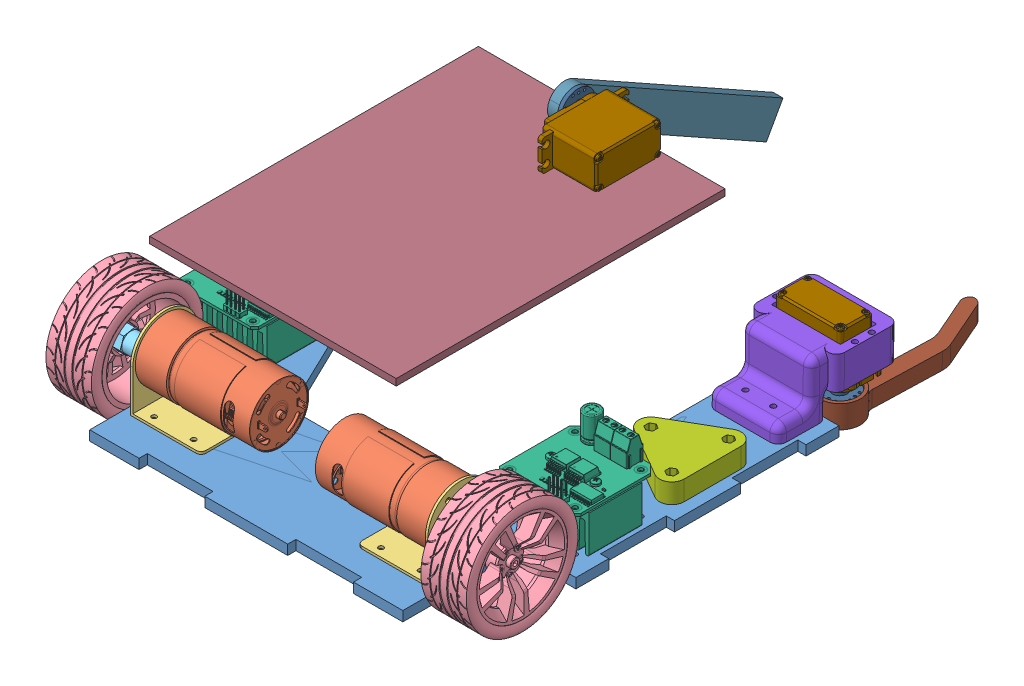
SolidWorks assembly Assem1, configuration Default. Lengths in mm.
Overall size (282.51 155.39 348.37).
30 component instances, 14 part files, 41 mates.
Components (placement in the parent):
- Part2-1: Part2 [Default] at (65.9546 135.2109 209.7386) size (261.02 6 230)
- assemblage_motor_complet-1: assemblage_motor_complet [Default] at (115.1812 215.9173 341.5945) x (0 0 -1) z (-1 0 0) size (92.56 92.56 113.78)
  - Motor 300RPM-1: Motor 300RPM [Default] at (60.9586 47.2064 18.9845) size (37 37 94.88)
  - BAse-motor-1: BAse-motor [Predeterminado] at (28.5836 74.7064 94.3595) x (1 0 0) z (0 0 -1) size (40 46 43)
  - wheel-1: wheel [Default] at (48.5836 55.7064 86.8847) x (-0.872522 -0.488575 0) z (-0.488575 0.872522 0) size (68 29.75 68)
  - accoupelement court-1: accoupelement court [Default] at (48.5836 55.7064 101.8595) x (-0.320714 0.947176 0) z (0 0 1) size (13.86 12 18)
- assemblage_motor_complet-2: assemblage_motor_complet [Default] at (107.4867 215.9173 244.4273) x (0 0 1) z (1 0 0) size (92.56 92.56 113.78)
  - Motor 300RPM-1: Motor 300RPM [Default] at (60.9586 47.2064 18.9845) size (37 37 94.88)
  - BAse-motor-1: BAse-motor [Predeterminado] at (28.5836 74.7064 94.3595) x (1 0 0) z (0 0 -1) size (40 46 43)
  - wheel-1: wheel [Default] at (48.5836 55.7064 86.8847) x (-0.872522 -0.488575 0) z (-0.488575 0.872522 0) size (68 29.75 68)
  - accoupelement court-1: accoupelement court [Default] at (48.5836 55.7064 101.8595) x (-0.320714 0.947176 0) z (0 0 1) size (13.86 12 18)
- IBT-2-module-only-1: IBT-2-module-only [Default] at (209.3463 164.2109 229.8359) size (51 40.62 49.7)
- IBT-2-module-only-4: IBT-2-module-only [Default] at (13.3217 164.5716 229.8359) size (51 40.62 49.7)
- gfg-1: gfg [Défaut] at (217.3463 141.2109 172.8314) x (0.866025 0 0.5) z (-0.5 0 0.866025) size (49.64 15.5 45)
- gfg-2: gfg [Défaut] at (5.3217 141.2109 172.8314) x (0.866025 0 -0.5) z (0.5 0 0.866025) size (49.64 15.5 45)
- support_servo_pince_lamen_isar-1: support_servo_pince_lamen_isar [Default] at (9.3217 155.972 83.8247) x (0 -0.01251 -0.999922) z (0 0.999922 -0.01251) size (68 53 35)
- Part2-2: Part2 [Default] at (65.9546 135.2109 209.7386) size (261.02 6 230)
- support_servo_pince_lamen_isar-2: support_servo_pince_lamen_isar [Default] at (213.3463 155.972 83.8247) x (0 -0.01251 -0.999922) z (0 0.999922 -0.01251) size (68 53 35)
- Servo noir-2: Servo noir [По умолчанию] at (9.3217 182.4699 83.4932) x (1 0 0) z (0 -0.01251 -0.999922) size (53 41.52 20)
- piece de liaison cercle MG996r-3: piece de liaison cercle MG996r [Défaut] at (-0.6783 141.3231 84.008) x (0.979866 0.002498 0.199641) z (0 -0.999922 0.01251) size (20.75 20.75 5.3)
- pince lamen-2: pince lamen [Default] at (-0.6783 134.0237 84.0993) x (0.02377 -0.012506 -0.999639) z (0 0.999922 -0.01251) size (105.33 28.11 13.75)
- Servo noir-3: Servo noir [По умолчанию] at (213.3463 182.4699 83.4932) x (-1 0 0) z (0 0.01251 0.999922) size (53 41.52 20)
- piece de liaison cercle MG996r-4: piece de liaison cercle MG996r [Défaut] at (223.3463 141.3231 84.008) x (-0.987212 0.001994 0.159399) z (0 -0.999922 0.01251) size (20.75 20.75 5.3)
- pince lamen-3: pince lamen [Default] at (223.3463 134.0237 84.0993) x (0.017139 -0.012508 -0.999775) z (0 -0.999922 0.01251) size (105.33 28.11 13.75)
- BillePorteuse-1: BillePorteuse [Défaut] at (5.3217 135.7109 172.8314) x (-1 0 0) z (0 0 1) size (31 21.5 31)
- BillePorteuse-2: BillePorteuse [Défaut] at (217.3463 135.7109 172.8314) x (-1 0 0) z (0 0 1) size (31 21.5 31)
- etage-1: etage [Default] at (111.334 241.2109 216.8002) x (0 0 -1) z (0 1 0) size (200 150 4)
- Servo noir-4: Servo noir [По умолчанию] at (150.296 255.2109 139.0433) x (0 0 1) z (0 -1 0) size (53 41.52 20)
- pince-1: pince [Default] at (100.996 223.6233 72.6584) x (0 -0.488677 -0.872465) z (1 0 0) size (150 20.75 6)
- piece de liaison cercle MG996r-5: piece de liaison cercle MG996r [Défaut] at (109.296 255.2109 129.0433) x (0 0.998874 -0.047442) z (-1 0 0) size (20.75 20.75 5.3)
Mates (geometry in assembly coordinates):
- Coincident5: coincident anti-aligned: plane of Part2-1 through (65.9546 141.2109 209.7386) normal (0 1 0); plane of assemblage_motor_complet-1/BAse motor-1 through (22.3217 141.2109 313.0109) normal (0 -1 0)
- Distance2: distance = 40 mm aligned: plane of Part2-1 through (-19.1783 141.2109 133.0109) normal (-1 0 0); plane of assemblage_motor_complet-1/BAse motor-1 through (20.8217 167.2109 293.0109) normal (-1 0 0)
- Distance1: distance = 20 mm aligned: plane of assemblage_motor_complet-1/BAse motor-1 through (22.3217 141.2109 313.0109) normal (0 0 1); plane of Part2-1 through (-19.1783 141.2109 333.0109) normal (0 0 1)
- Distance3: distance = 7 mm aligned: plane of IBT-2 (module only)-1 through (234.8463 164.2109 248.0109) normal (1 0 0); plane of Part2-1 through (241.8463 141.2109 133.0109) normal (1 0 0)
- Distance4: distance = 15 mm aligned: plane of IBT-2 (module only)-1 through (209.3463 164.2109 248.0109) normal (0 0 1); plane of Part2-1 through (65.9546 131.2109 263.0109) normal (0 0 1)
- Coincident12: coincident: plane of Part2-1 through (65.9546 141.2109 209.7386) normal (0 1 0); point of IBT-2 (module only)-1
- Distance5: distance = 7 mm aligned: plane of IBT-2 (module only)-4 through (-12.1783 164.5716 248.0109) normal (-1 0 0); plane of Part2-1 through (-19.1783 141.2109 133.0109) normal (-1 0 0)
- Distance6: distance = 15 mm aligned: plane of IBT-2 (module only)-4 through (13.3217 164.5716 248.0109) normal (0 0 1); plane of Part2-1 through (-19.1783 131.2109 263.0109) normal (0 0 1)
- Distance10: distance = 7 mm aligned: plane of gfg-1 through (234.8463 153.2109 155.5109) normal (1 0 0); plane of Part2-1 through (241.8463 141.2109 133.0109) normal (1 0 0)
- Distance11: distance = 45 mm: cylinder of gfg-1 through (227.3463 153.2109 155.5109) axis (0 -1 0) radius 7.5; plane of Part2-1 through (65.9546 135.2109 103.0109) normal (0 0 -1)
- Coincident24: coincident anti-aligned: plane of Servo noir-1 through (-18.4913 420.0414 279.4883) normal (0 0 1); plane of support_servo_pince_lamen_isar-3 through (-10.8029 395.353 279.4883) normal (0 0 -1)
- Width1: width anti-aligned: plane of Servo noir-1 through (-20.8029 413.353 273.4883) normal (-1 0 0); plane of Servo noir-1 through (-0.8029 413.353 273.4883) normal (1 0 0); plane of support_servo_pince_lamen_isar-3 through (-21.8029 374.353 299.4883) normal (1 0 0); plane of support_servo_pince_lamen_isar-3 through (0.1971 374.353 299.4883) normal (-1 0 0)
- Coincident29: coincident aligned: circle of Servo noir-2; circle of piece de liaison cercle MG996r-3
- Coincident30: coincident anti-aligned: plane of support_servo_pince_lamen_isar-1 through (9.3217 155.972 83.8247) normal (0 -0.999922 0.01251); plane of Servo noir-2 through (-15.3667 156.0682 91.5125) normal (0 0.999922 -0.01251)
- Coincident31: coincident aligned: circle of piece de liaison cercle MG996r-3; circle of pince lamen-2
- Coincident32: coincident aligned: circle of piece de liaison cercle MG996r-3; circle of pince lamen-2
- Concentric10: concentric aligned: circle of support_servo_pince_lamen_isar-1; circle of Servo noir-2
- Concentric11: concentric aligned: circle of support_servo_pince_lamen_isar-1; circle of Servo noir-2
- Concentric12: concentric aligned: circle of support_servo_pince_lamen_isar-2; circle of Servo noir-3
- Concentric13: concentric aligned: circle of support_servo_pince_lamen_isar-2; circle of Servo noir-3
- Coincident33: coincident anti-aligned: plane of support_servo_pince_lamen_isar-2 through (213.3463 155.972 83.8247) normal (0 -0.999922 0.01251); plane of Servo noir-3 through (238.0347 155.8758 76.1369) normal (0 0.999922 -0.01251)
- Coincident35: coincident aligned: circle of Servo noir-3; circle of piece de liaison cercle MG996r-4
- Coincident36: coincident anti-aligned: circle of piece de liaison cercle MG996r-4; circle of pince lamen-3
- Coincident37: coincident anti-aligned: circle of piece de liaison cercle MG996r-4; circle of pince lamen-3
- Distance12: distance = 7 mm aligned: plane of support_servo_pince_lamen_isar-1 through (-12.1783 176.5834 132.5707) normal (-1 0 0); plane of Part2-1 through (-19.1783 141.2109 133.0109) normal (-1 0 0)
- Distance13: distance = 0 mm: line of support_servo_pince_lamen_isar-1 through (-7.1783 141.2109 103.0109) axis (1 0 0); line of Part2-2 through (-19.1783 141.2109 103.0109) axis (1 0 0)
- Coincident41: coincident anti-aligned: plane of Part2-1 through (65.9546 141.2109 209.7386) normal (0 1 0); plane of gfg-1 through (227.3463 141.2109 155.5109) normal (0 -1 0)
- Concentric14: concentric aligned: cylinder of gfg-2 through (5.3217 153.2109 172.8314) axis (0 -1 0) radius 11.9; cylinder of BillePorteuse-1 through (5.3217 128.2109 172.8314) axis (0 -1 0) radius 12
- Coincident42: coincident anti-aligned: plane of gfg-2 through (5.3217 137.7109 172.8314) normal (0 -1 0); plane of BillePorteuse-1 through (17.3217 137.7109 172.8314) normal (0 1 0)
- Concentric15: concentric aligned: cylinder of gfg-1 through (217.3463 153.2109 172.8314) axis (0 -1 0) radius 11.9; cylinder of BillePorteuse-2 through (217.3463 128.2109 172.8314) axis (0 -1 0) radius 12
- Coincident43: coincident anti-aligned: plane of gfg-1 through (217.3463 137.7109 172.8314) normal (0 -1 0); plane of BillePorteuse-2 through (229.3463 137.7109 172.8314) normal (0 1 0)
- Parallel1: parallel anti-aligned: plane of Part2-1 through (65.9546 141.2109 209.7386) normal (0 1 0); plane of etage-1 through (111.334 241.2109 216.8002) normal (0 -1 0)
- Parallel2: parallel aligned: plane of Part2-1 through (-19.1783 141.2109 333.0109) normal (0 0 1); plane of etage-1 through (36.334 245.2109 316.8002) normal (0 0 1)
- Width2: width anti-aligned: plane of etage-1 through (186.334 245.2109 316.8002) normal (1 0 0); plane of Part2-1 through (36.334 245.2109 316.8002) normal (-1 0 0); plane of etage-1 through (16.109 131.2109 333.0109) normal (-1 0 0); plane of Part2-1 through (206.559 131.2109 209.7386) normal (1 0 0)
- Coincident46: coincident: plane of etage-1 through (111.334 245.2109 216.8002) normal (0 1 0); plane of Servo noir-4 through (117.796 245.2109 121.0433) normal (0 -1 0)
- Parallel3: parallel aligned: plane of etage-1 through (186.334 245.2109 316.8002) normal (1 0 0); plane of Servo noir-4 through (150.296 247.2109 121.0433) normal (1 0 0)
- Distance14: distance = 100 mm: plane of etage-1 through (111.334 241.2109 216.8002) normal (0 -1 0); plane of Part2-1 through (65.9546 141.2109 209.7386) normal (0 1 0)
- Concentric16: concentric anti-aligned: cylinder of Servo noir-4 through (108.796 255.2109 129.0433) axis (1 0 0) radius 3; cylinder of piece de liaison cercle MG996r-5 through (112.296 255.2109 129.0433) axis (-1 0 0) radius 4.4
- Coincident49: coincident anti-aligned: circle of Servo noir-4; plane of piece de liaison cercle MG996r-5 through (112.296 255.2109 129.0433) normal (1 0 0)
- Concentric17: concentric anti-aligned: cylinder of pince-1 through (106.996 255.2109 129.0433) axis (-1 0 0) radius 10.37; cylinder of piece de liaison cercle MG996r-5 through (106.996 255.2109 129.0433) axis (1 0 0) radius 10.375
- Coincident50: coincident anti-aligned: plane of pince-1 through (106.996 255.2021 129.0482) normal (1 0 0); plane of piece de liaison cercle MG996r-5 through (106.996 255.2109 129.0433) normal (-1 0 0)
